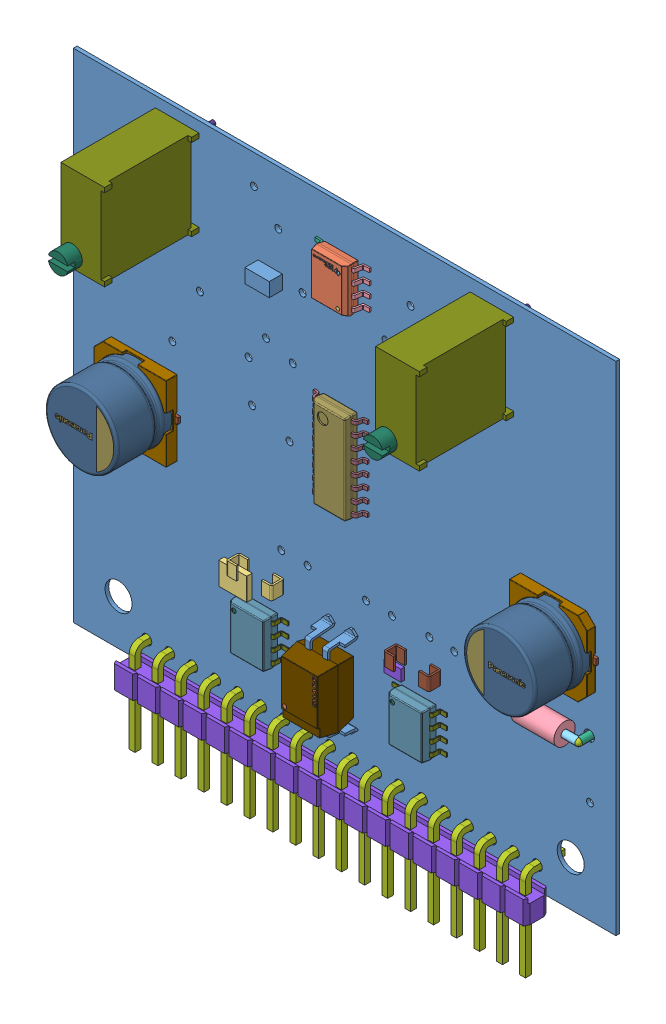
SolidWorks assembly PWM_controller, configuration Default. Lengths in mm.
Overall size (60 62.62 16.05).
432 component instances, 52 part files, 0 mates.
Components (placement in the parent):
- PWM_controller.step-2: PWM_controller.step [Default] at origin size (60 62.62 16.05)
  - Board.step-1: Board.step [Default] at origin size (60 55 0.41)
    - Open CASCADE STEP translator 6.8 2.1.1.step-1: Open CASCADE STEP translator 6.8 2.1.1.step [Default] at (0 0 -0.4115) size (60 55 0.41)
  - R32.step-1: R32.step [Default] at origin size (3.2 2.5 0.7)
    - Res_Stackpole_Electronics_RMCF1210JT5K10_eec.step-1: Res_Stackpole_Electronics_RMCF1210JT5K10_eec.step [Default] at (249.8598 58.1914 -0.4115) x (-1 0 0) z (0 0 -1) size (3.2 2.5 0.7)
      - terminals.step-1: terminals.step [Default] at origin size (3.2 2.5 0.7)
      - body.step-1: body.step [Default] at origin size (3.1 2.5 0.6)
      - top.step-1: top.step [Default] at (-0.71 0 0.65) size (2.2 2.5 0.05)
      - logo.step-1: logo.step [Default] at (0 0 0.7) size (1.25 0.57 0)
  - C2.step-1: C2.step [Default] at origin size (2.7 3.4 1)
    - 6948496496.step-1: 6948496496.step [Default] at (219.9386 58.9514 -1.4115) size (2.7 0.5 1)
      - Extruded.step-1: Extruded.step [Default] at origin size (2.7 0.5 1)
    - 6948496496.step-2: 6948496496.step [Default] at (219.9386 61.8514 -1.4115) size (2.7 0.5 1)
      - Extruded.step-1: Extruded.step [Default] at origin size (2.7 0.5 1)
    - 6948486416.step-1: 6948486416.step [Default] at (219.9386 60.4014 -1.4115) size (2.7 2.4 1)
      - Extruded-0.step-1: Extruded-0.step [Default] at origin size (2.7 2.4 1)
  - C1.step-1: C1.step [Default] at origin size (2.7 3.4 1)
    - 6948496496.step-1: 6948496496.step [Default] at (237.0328 57.9862 -1.4115) size (2.7 0.5 1)
      - Extruded.step-1: Extruded.step [Default] at origin size (2.7 0.5 1)
    - 6948496496.step-2: 6948496496.step [Default] at (237.0328 60.8862 -1.4115) size (2.7 0.5 1)
      - Extruded.step-1: Extruded.step [Default] at origin size (2.7 0.5 1)
    - 6948486416.step-1: 6948486416.step [Default] at (237.0328 59.4362 -1.4115) size (2.7 2.4 1)
      - Extruded-0.step-1: Extruded-0.step [Default] at origin size (2.7 2.4 1)
  - R31.step-1: R31.step [Default] at origin size (1.25 2 0.5)
    - Res_Vishay_CRCW0805100KFKEA_eec.step-1: Res_Vishay_CRCW0805100KFKEA_eec.step [Default] at (205.232 89.4842 -0.4115) x (0 1 0) z (0 0 -1) size (2 1.25 0.5)
      - body-1.step-1: body-1.step [Default] at (0 0 0.45) x (1 0 0) z (0 0 -1) size (1.9 1.25 0.4)
      - pad.step-1: pad.step [Default] at (-0.8133 -0.625 0.5) x (1 0 0) z (0 1 0) size (0.3 0.5 1.25)
      - pad.step-2: pad.step [Default] at (0.8133 0.625 0.5) x (-1 0 0) z (0 -1 0) size (0.3 0.5 1.25)
      - top-2.step-1: top-2.step [Default] at (0 0 0.05) x (1 0 0) z (0 0 -1) size (1.4 1.25 0.05)
      - top-2.step-2: top-2.step [Default] at (0 0 0.5) x (1 0 0) z (0 0 -1) size (1.4 1.25 0.05)
      - Vishay.step-1: Vishay.step [Default] at (0.032 -0.7832 0.5) size (0.44 0.37 0)
  - R4.step-1: R4.step [Default] at origin size (1.25 2 0.5)
    - Res_Vishay_CRCW0805100KFKEA_eec.step-1: Res_Vishay_CRCW0805100KFKEA_eec.step [Default] at (206.9846 87.503 -0.4115) x (0 -1 0) z (0 0 -1) size (2 1.25 0.5)
      - body-1.step-1: body-1.step [Default] at (0 0 0.45) x (1 0 0) z (0 0 -1) size (1.9 1.25 0.4)
      - pad.step-1: pad.step [Default] at (-0.8133 -0.625 0.5) x (1 0 0) z (0 1 0) size (0.3 0.5 1.25)
      - pad.step-2: pad.step [Default] at (0.8133 0.625 0.5) x (-1 0 0) z (0 -1 0) size (0.3 0.5 1.25)
      - top-2.step-1: top-2.step [Default] at (0 0 0.05) x (1 0 0) z (0 0 -1) size (1.4 1.25 0.05)
      - top-2.step-2: top-2.step [Default] at (0 0 0.5) x (1 0 0) z (0 0 -1) size (1.4 1.25 0.05)
      - Vishay.step-1: Vishay.step [Default] at (0.032 -0.7832 0.5) size (0.44 0.37 0)
  - R3.step-1: R3.step [Default] at origin size (1.25 2 0.5)
    - Res_Vishay_CRCW0805100KFKEA_eec.step-1: Res_Vishay_CRCW0805100KFKEA_eec.step [Default] at (210.3628 76.8604 -0.4115) x (0 -1 0) z (0 0 -1) size (2 1.25 0.5)
      - body-1.step-1: body-1.step [Default] at (0 0 0.45) x (1 0 0) z (0 0 -1) size (1.9 1.25 0.4)
      - pad.step-1: pad.step [Default] at (-0.8133 -0.625 0.5) x (1 0 0) z (0 1 0) size (0.3 0.5 1.25)
      - pad.step-2: pad.step [Default] at (0.8133 0.625 0.5) x (-1 0 0) z (0 -1 0) size (0.3 0.5 1.25)
      - top-2.step-1: top-2.step [Default] at (0 0 0.05) x (1 0 0) z (0 0 -1) size (1.4 1.25 0.05)
      - top-2.step-2: top-2.step [Default] at (0 0 0.5) x (1 0 0) z (0 0 -1) size (1.4 1.25 0.05)
      - Vishay.step-1: Vishay.step [Default] at (0.032 -0.7832 0.5) size (0.44 0.37 0)
  - R2.step-1: R2.step [Default] at origin size (1.25 2 0.5)
    - Res_Vishay_CRCW0805100KFKEA_eec.step-1: Res_Vishay_CRCW0805100KFKEA_eec.step [Default] at (223.7232 76.7588 -0.4115) x (0 -1 0) z (0 0 -1) size (2 1.25 0.5)
      - body-1.step-1: body-1.step [Default] at (0 0 0.45) x (1 0 0) z (0 0 -1) size (1.9 1.25 0.4)
      - pad.step-1: pad.step [Default] at (-0.8133 -0.625 0.5) x (1 0 0) z (0 1 0) size (0.3 0.5 1.25)
      - pad.step-2: pad.step [Default] at (0.8133 0.625 0.5) x (-1 0 0) z (0 -1 0) size (0.3 0.5 1.25)
      - top-2.step-1: top-2.step [Default] at (0 0 0.05) x (1 0 0) z (0 0 -1) size (1.4 1.25 0.05)
      - top-2.step-2: top-2.step [Default] at (0 0 0.5) x (1 0 0) z (0 0 -1) size (1.4 1.25 0.05)
      - Vishay.step-1: Vishay.step [Default] at (0.032 -0.7832 0.5) size (0.44 0.37 0)
  - R1.step-1: R1.step [Default] at origin size (1.25 2 0.5)
    - Res_Vishay_CRCW0805100KFKEA_eec.step-1: Res_Vishay_CRCW0805100KFKEA_eec.step [Default] at (225.7044 76.7842 -0.4115) x (0 1 0) z (0 0 -1) size (2 1.25 0.5)
      - body-1.step-1: body-1.step [Default] at (0 0 0.45) x (1 0 0) z (0 0 -1) size (1.9 1.25 0.4)
      - pad.step-1: pad.step [Default] at (-0.8133 -0.625 0.5) x (1 0 0) z (0 1 0) size (0.3 0.5 1.25)
      - pad.step-2: pad.step [Default] at (0.8133 0.625 0.5) x (-1 0 0) z (0 -1 0) size (0.3 0.5 1.25)
      - top-2.step-1: top-2.step [Default] at (0 0 0.05) x (1 0 0) z (0 0 -1) size (1.4 1.25 0.05)
      - top-2.step-2: top-2.step [Default] at (0 0 0.5) x (1 0 0) z (0 0 -1) size (1.4 1.25 0.05)
      - Vishay.step-1: Vishay.step [Default] at (0.032 -0.7832 0.5) size (0.44 0.37 0)
  - R30.step-1: R30.step [Default] at origin size (1.25 2 0.5)
    - Res_Vishay_CRCW0805100KFKEA_eec.step-1: Res_Vishay_CRCW0805100KFKEA_eec.step [Default] at (220.9546 82.6008 -0.4115) x (0 -1 0) z (0 0 -1) size (2 1.25 0.5)
      - body-1.step-1: body-1.step [Default] at (0 0 0.45) x (1 0 0) z (0 0 -1) size (1.9 1.25 0.4)
      - pad.step-1: pad.step [Default] at (-0.8133 -0.625 0.5) x (1 0 0) z (0 1 0) size (0.3 0.5 1.25)
      - pad.step-2: pad.step [Default] at (0.8133 0.625 0.5) x (-1 0 0) z (0 -1 0) size (0.3 0.5 1.25)
      - top-2.step-1: top-2.step [Default] at (0 0 0.05) x (1 0 0) z (0 0 -1) size (1.4 1.25 0.05)
      - top-2.step-2: top-2.step [Default] at (0 0 0.5) x (1 0 0) z (0 0 -1) size (1.4 1.25 0.05)
      - Vishay.step-1: Vishay.step [Default] at (0.032 -0.7832 0.5) size (0.44 0.37 0)
  - R29.step-1: R29.step [Default] at origin size (1.25 2 0.5)
    - Res_Vishay_CRCW0805100KFKEA_eec.step-1: Res_Vishay_CRCW0805100KFKEA_eec.step [Default] at (211.2772 90.4084 -0.4115) x (0 -1 0) z (0 0 -1) size (2 1.25 0.5)
      - body-1.step-1: body-1.step [Default] at (0 0 0.45) x (1 0 0) z (0 0 -1) size (1.9 1.25 0.4)
      - pad.step-1: pad.step [Default] at (-0.8133 -0.625 0.5) x (1 0 0) z (0 1 0) size (0.3 0.5 1.25)
      - pad.step-2: pad.step [Default] at (0.8133 0.625 0.5) x (-1 0 0) z (0 -1 0) size (0.3 0.5 1.25)
      - top-2.step-1: top-2.step [Default] at (0 0 0.05) x (1 0 0) z (0 0 -1) size (1.4 1.25 0.05)
      - top-2.step-2: top-2.step [Default] at (0 0 0.5) x (1 0 0) z (0 0 -1) size (1.4 1.25 0.05)
      - Vishay.step-1: Vishay.step [Default] at (0.032 -0.7832 0.5) size (0.44 0.37 0)
  - R28.step-1: R28.step [Default] at origin size (2 1.25 0.5)
    - Res_Vishay_CRCW0805100KFKEA_eec.step-1: Res_Vishay_CRCW0805100KFKEA_eec.step [Default] at (224.0026 85.6742 -0.4115) x (-1 0 0) z (0 0 -1) size (2 1.25 0.5)
      - body-1.step-1: body-1.step [Default] at (0 0 0.45) x (1 0 0) z (0 0 -1) size (1.9 1.25 0.4)
      - pad.step-1: pad.step [Default] at (-0.8133 -0.625 0.5) x (1 0 0) z (0 1 0) size (0.3 0.5 1.25)
      - pad.step-2: pad.step [Default] at (0.8133 0.625 0.5) x (-1 0 0) z (0 -1 0) size (0.3 0.5 1.25)
      - top-2.step-1: top-2.step [Default] at (0 0 0.05) x (1 0 0) z (0 0 -1) size (1.4 1.25 0.05)
      - top-2.step-2: top-2.step [Default] at (0 0 0.5) x (1 0 0) z (0 0 -1) size (1.4 1.25 0.05)
      - Vishay.step-1: Vishay.step [Default] at (0.032 -0.7832 0.5) size (0.44 0.37 0)
  - R27.step-1: R27.step [Default] at origin size (1.25 2 0.5)
    - Res_Vishay_CRCW0805100KFKEA_eec.step-1: Res_Vishay_CRCW0805100KFKEA_eec.step [Default] at (213.7156 87.5792 -0.4115) x (0 -1 0) z (0 0 -1) size (2 1.25 0.5)
      - body-1.step-1: body-1.step [Default] at (0 0 0.45) x (1 0 0) z (0 0 -1) size (1.9 1.25 0.4)
      - pad.step-1: pad.step [Default] at (-0.8133 -0.625 0.5) x (1 0 0) z (0 1 0) size (0.3 0.5 1.25)
      - pad.step-2: pad.step [Default] at (0.8133 0.625 0.5) x (-1 0 0) z (0 -1 0) size (0.3 0.5 1.25)
      - top-2.step-1: top-2.step [Default] at (0 0 0.05) x (1 0 0) z (0 0 -1) size (1.4 1.25 0.05)
      - top-2.step-2: top-2.step [Default] at (0 0 0.5) x (1 0 0) z (0 0 -1) size (1.4 1.25 0.05)
      - Vishay.step-1: Vishay.step [Default] at (0.032 -0.7832 0.5) size (0.44 0.37 0)
  - C14.step-1: C14.step [Default] at origin size (1.25 2 0.88)
    - Cap_KEMET_C0805C472J3HAC_eec.step-1: Cap_KEMET_C0805C472J3HAC_eec.step [Default] at (211.2264 84.3788 -0.4115) x (0 1 0) z (0 0 -1) size (1 1.15 0.78)
    - Cap_KEMET_C0805C472J3HAC_eec-3.step-1: Cap_KEMET_C0805C472J3HAC_eec-3.step [Default] at (211.2264 84.3788 -0.4115) x (0 1 0) z (0 0 -1) size (2 1.25 0.88)
    - Cap_KEMET_C0805C472J3HAC_eec-4.step-1: Cap_KEMET_C0805C472J3HAC_eec-4.step [Default] at (211.2264 84.3788 -0.4115) x (0 1 0) z (0 0 -1) size (0.59 0.12 0)
  - C13.step-1: C13.step [Default] at origin size (1.25 2 0.88)
    - Cap_KEMET_C0805C472J3HAC_eec.step-1: Cap_KEMET_C0805C472J3HAC_eec.step [Default] at (213.6648 84.3788 -0.4115) x (0 -1 0) z (0 0 -1) size (1 1.15 0.78)
    - Cap_KEMET_C0805C472J3HAC_eec-3.step-1: Cap_KEMET_C0805C472J3HAC_eec-3.step [Default] at (213.6648 84.3788 -0.4115) x (0 -1 0) z (0 0 -1) size (2 1.25 0.88)
    - Cap_KEMET_C0805C472J3HAC_eec-4.step-1: Cap_KEMET_C0805C472J3HAC_eec-4.step [Default] at (213.6648 84.3788 -0.4115) x (0 -1 0) z (0 0 -1) size (0.59 0.12 0)
  - R21.step-1: R21.step [Default] at origin size (2 1.25 0.5)
    - Res_Vishay_CRCW0805100KFKEA_eec.step-1: Res_Vishay_CRCW0805100KFKEA_eec.step [Default] at (225.0694 92.8624 -0.4115) x (1 0 0) z (0 0 -1) size (2 1.25 0.5)
      - body-1.step-1: body-1.step [Default] at (0 0 0.45) x (1 0 0) z (0 0 -1) size (1.9 1.25 0.4)
      - pad.step-1: pad.step [Default] at (-0.8133 -0.625 0.5) x (1 0 0) z (0 1 0) size (0.3 0.5 1.25)
      - pad.step-2: pad.step [Default] at (0.8133 0.625 0.5) x (-1 0 0) z (0 -1 0) size (0.3 0.5 1.25)
      - top-2.step-1: top-2.step [Default] at (0 0 0.05) x (1 0 0) z (0 0 -1) size (1.4 1.25 0.05)
      - top-2.step-2: top-2.step [Default] at (0 0 0.5) x (1 0 0) z (0 0 -1) size (1.4 1.25 0.05)
      - Vishay.step-1: Vishay.step [Default] at (0.032 -0.7832 0.5) size (0.44 0.37 0)
  - R20.step-1: R20.step [Default] at origin size (1.25 2 0.5)
    - Res_Vishay_CRCW0805100KFKEA_eec.step-1: Res_Vishay_CRCW0805100KFKEA_eec.step [Default] at (216.7382 97.3074 -0.4115) x (0 -1 0) z (0 0 -1) size (2 1.25 0.5)
      - body-1.step-1: body-1.step [Default] at (0 0 0.45) x (1 0 0) z (0 0 -1) size (1.9 1.25 0.4)
      - pad.step-1: pad.step [Default] at (-0.8133 -0.625 0.5) x (1 0 0) z (0 1 0) size (0.3 0.5 1.25)
      - pad.step-2: pad.step [Default] at (0.8133 0.625 0.5) x (-1 0 0) z (0 -1 0) size (0.3 0.5 1.25)
      - top-2.step-1: top-2.step [Default] at (0 0 0.05) x (1 0 0) z (0 0 -1) size (1.4 1.25 0.05)
      - top-2.step-2: top-2.step [Default] at (0 0 0.5) x (1 0 0) z (0 0 -1) size (1.4 1.25 0.05)
      - Vishay.step-1: Vishay.step [Default] at (0.032 -0.7832 0.5) size (0.44 0.37 0)
  - R19.step-1: R19.step [Default] at origin size (4.83 9.53 16.05)
    - Res_Bourns_3296W-1-504LF_eec.step-1: Res_Bourns_3296W-1-504LF_eec.step [Default] at (210.3653 92.9274 10.0159) x (0 0 -1) z (-1 0 0) size (1.59 2.18 2.18)
    - Res_Bourns_3296W-1-504LF_eec-5.step-1: Res_Bourns_3296W-1-504LF_eec-5.step [Default] at (210.3653 92.9274 10.0159) x (0 0 -1) z (-1 0 0) size (10.46 9.53 4.83)
    - Res_Bourns_3296W-1-504LF_eec-6.step-1: Res_Bourns_3296W-1-504LF_eec-6.step [Default] at (210.3653 92.9274 10.0159) x (0 0 -1) z (-1 0 0) size (4.53 5.59 0.51)
    - Res_Bourns_3296W-1-504LF_eec-7.step-1: Res_Bourns_3296W-1-504LF_eec-7.step [Default] at (210.3653 92.9274 10.0159) x (0 0 -1) z (-1 0 0) size (0.78 6.02 0.01)
  - R18.step-1: R18.step [Default] at origin size (1.25 2 0.5)
    - Res_Vishay_CRCW0805100KFKEA_eec.step-1: Res_Vishay_CRCW0805100KFKEA_eec.step [Default] at (214.884 97.3328 -0.4115) x (0 -1 0) z (0 0 -1) size (2 1.25 0.5)
      - body-1.step-1: body-1.step [Default] at (0 0 0.45) x (1 0 0) z (0 0 -1) size (1.9 1.25 0.4)
      - pad.step-1: pad.step [Default] at (-0.8133 -0.625 0.5) x (1 0 0) z (0 1 0) size (0.3 0.5 1.25)
      - pad.step-2: pad.step [Default] at (0.8133 0.625 0.5) x (-1 0 0) z (0 -1 0) size (0.3 0.5 1.25)
      - top-2.step-1: top-2.step [Default] at (0 0 0.05) x (1 0 0) z (0 0 -1) size (1.4 1.25 0.05)
      - top-2.step-2: top-2.step [Default] at (0 0 0.5) x (1 0 0) z (0 0 -1) size (1.4 1.25 0.05)
      - Vishay.step-1: Vishay.step [Default] at (0.032 -0.7832 0.5) size (0.44 0.37 0)
  - R17.step-1: R17.step [Default] at origin size (2 1.25 0.5)
    - Res_Vishay_CRCW0805100KFKEA_eec.step-1: Res_Vishay_CRCW0805100KFKEA_eec.step [Default] at (222.631 97.6376 -0.4115) x (-1 0 0) z (0 0 -1) size (2 1.25 0.5)
      - body-1.step-1: body-1.step [Default] at (0 0 0.45) x (1 0 0) z (0 0 -1) size (1.9 1.25 0.4)
      - pad.step-1: pad.step [Default] at (-0.8133 -0.625 0.5) x (1 0 0) z (0 1 0) size (0.3 0.5 1.25)
      - pad.step-2: pad.step [Default] at (0.8133 0.625 0.5) x (-1 0 0) z (0 -1 0) size (0.3 0.5 1.25)
      - top-2.step-1: top-2.step [Default] at (0 0 0.05) x (1 0 0) z (0 0 -1) size (1.4 1.25 0.05)
      - top-2.step-2: top-2.step [Default] at (0 0 0.5) x (1 0 0) z (0 0 -1) size (1.4 1.25 0.05)
      - Vishay.step-1: Vishay.step [Default] at (0.032 -0.7832 0.5) size (0.44 0.37 0)
  - D5.step-1: D5.step [Default] at origin size (2.7 1.55 1.45)
    - 6038362448.step-1: 6038362448.step [Default] at (235.0262 92.964 0) size (2.7 1.55 1.45)
      - Extruded-8.step-1: Extruded-8.step [Default] at origin size (2.7 1.55 1.45)
  - D4.step-1: D4.step [Default] at origin size (2.7 1.55 1.45)
    - 6038362448.step-1: 6038362448.step [Default] at (218.6178 92.7862 0) size (2.7 1.55 1.45)
      - Extruded-8.step-1: Extruded-8.step [Default] at origin size (2.7 1.55 1.45)
  - C12.step-1: C12.step [Default] at origin size (2 1.25 0.88)
    - Cap_KEMET_C0805C472J3HAC_eec.step-1: Cap_KEMET_C0805C472J3HAC_eec.step [Default] at (237.2614 97.9424 -0.4115) x (1 0 0) z (0 0 -1) size (1 1.15 0.78)
    - Cap_KEMET_C0805C472J3HAC_eec-3.step-1: Cap_KEMET_C0805C472J3HAC_eec-3.step [Default] at (237.2614 97.9424 -0.4115) x (1 0 0) z (0 0 -1) size (2 1.25 0.88)
    - Cap_KEMET_C0805C472J3HAC_eec-4.step-1: Cap_KEMET_C0805C472J3HAC_eec-4.step [Default] at (237.2614 97.9424 -0.4115) x (1 0 0) z (0 0 -1) size (0.59 0.12 0)
  - C11.step-1: C11.step [Default] at origin size (1.25 2 0.88)
    - Cap_KEMET_C0805C472J3HAC_eec.step-1: Cap_KEMET_C0805C472J3HAC_eec.step [Default] at (212.6996 97.3836 -0.4115) x (0 -1 0) z (0 0 -1) size (1 1.15 0.78)
    - Cap_KEMET_C0805C472J3HAC_eec-3.step-1: Cap_KEMET_C0805C472J3HAC_eec-3.step [Default] at (212.6996 97.3836 -0.4115) x (0 -1 0) z (0 0 -1) size (2 1.25 0.88)
    - Cap_KEMET_C0805C472J3HAC_eec-4.step-1: Cap_KEMET_C0805C472J3HAC_eec-4.step [Default] at (212.6996 97.3836 -0.4115) x (0 -1 0) z (0 0 -1) size (0.59 0.12 0)
  - R25.step-1: R25.step [Default] at origin size (2 1.25 0.5)
    - Res_Vishay_CRCW0805100KFKEA_eec.step-1: Res_Vishay_CRCW0805100KFKEA_eec.step [Default] at (231.2416 97.663 -0.4115) x (-1 0 0) z (0 0 -1) size (2 1.25 0.5)
      - body-1.step-1: body-1.step [Default] at (0 0 0.45) x (1 0 0) z (0 0 -1) size (1.9 1.25 0.4)
      - pad.step-1: pad.step [Default] at (-0.8133 -0.625 0.5) x (1 0 0) z (0 1 0) size (0.3 0.5 1.25)
      - pad.step-2: pad.step [Default] at (0.8133 0.625 0.5) x (-1 0 0) z (0 -1 0) size (0.3 0.5 1.25)
      - top-2.step-1: top-2.step [Default] at (0 0 0.05) x (1 0 0) z (0 0 -1) size (1.4 1.25 0.05)
      - top-2.step-2: top-2.step [Default] at (0 0 0.5) x (1 0 0) z (0 0 -1) size (1.4 1.25 0.05)
      - Vishay.step-1: Vishay.step [Default] at (0.032 -0.7832 0.5) size (0.44 0.37 0)
  - R23.step-1: R23.step [Default] at origin size (2 1.25 0.5)
    - Res_Vishay_CRCW0805100KFKEA_eec.step-1: Res_Vishay_CRCW0805100KFKEA_eec.step [Default] at (237.2614 100.1268 -0.4115) x (1 0 0) z (0 0 -1) size (2 1.25 0.5)
      - body-1.step-1: body-1.step [Default] at (0 0 0.45) x (1 0 0) z (0 0 -1) size (1.9 1.25 0.4)
      - pad.step-1: pad.step [Default] at (-0.8133 -0.625 0.5) x (1 0 0) z (0 1 0) size (0.3 0.5 1.25)
      - pad.step-2: pad.step [Default] at (0.8133 0.625 0.5) x (-1 0 0) z (0 -1 0) size (0.3 0.5 1.25)
      - top-2.step-1: top-2.step [Default] at (0 0 0.05) x (1 0 0) z (0 0 -1) size (1.4 1.25 0.05)
      - top-2.step-2: top-2.step [Default] at (0 0 0.5) x (1 0 0) z (0 0 -1) size (1.4 1.25 0.05)
      - Vishay.step-1: Vishay.step [Default] at (0.032 -0.7832 0.5) size (0.44 0.37 0)
  - R26.step-1: R26.step [Default] at origin size (2 1.25 0.5)
    - Res_Vishay_CRCW0805100KFKEA_eec.step-1: Res_Vishay_CRCW0805100KFKEA_eec.step [Default] at (228.6508 92.8624 -0.4115) x (-1 0 0) z (0 0 -1) size (2 1.25 0.5)
      - body-1.step-1: body-1.step [Default] at (0 0 0.45) x (1 0 0) z (0 0 -1) size (1.9 1.25 0.4)
      - pad.step-1: pad.step [Default] at (-0.8133 -0.625 0.5) x (1 0 0) z (0 1 0) size (0.3 0.5 1.25)
      - pad.step-2: pad.step [Default] at (0.8133 0.625 0.5) x (-1 0 0) z (0 -1 0) size (0.3 0.5 1.25)
      - top-2.step-1: top-2.step [Default] at (0 0 0.05) x (1 0 0) z (0 0 -1) size (1.4 1.25 0.05)
      - top-2.step-2: top-2.step [Default] at (0 0 0.5) x (1 0 0) z (0 0 -1) size (1.4 1.25 0.05)
      - Vishay.step-1: Vishay.step [Default] at (0.032 -0.7832 0.5) size (0.44 0.37 0)
  - R22.step-1: R22.step [Default] at origin size (2 1.25 0.5)
    - Res_Vishay_CRCW0805100KFKEA_eec.step-1: Res_Vishay_CRCW0805100KFKEA_eec.step [Default] at (234.2388 95.2754 -0.4115) x (1 0 0) z (0 0 -1) size (2 1.25 0.5)
      - body-1.step-1: body-1.step [Default] at (0 0 0.45) x (1 0 0) z (0 0 -1) size (1.9 1.25 0.4)
      - pad.step-1: pad.step [Default] at (-0.8133 -0.625 0.5) x (1 0 0) z (0 1 0) size (0.3 0.5 1.25)
      - pad.step-2: pad.step [Default] at (0.8133 0.625 0.5) x (-1 0 0) z (0 -1 0) size (0.3 0.5 1.25)
      - top-2.step-1: top-2.step [Default] at (0 0 0.05) x (1 0 0) z (0 0 -1) size (1.4 1.25 0.05)
      - top-2.step-2: top-2.step [Default] at (0 0 0.5) x (1 0 0) z (0 0 -1) size (1.4 1.25 0.05)
      - Vishay.step-1: Vishay.step [Default] at (0.032 -0.7832 0.5) size (0.44 0.37 0)
  - R24.step-1: R24.step [Default] at origin size (4.83 9.53 16.05)
    - Res_Bourns_3296W-1-504LF_eec.step-1: Res_Bourns_3296W-1-504LF_eec.step [Default] at (245.1683 92.6988 10.0159) x (0 0 -1) z (-1 0 0) size (1.59 2.18 2.18)
    - Res_Bourns_3296W-1-504LF_eec-5.step-1: Res_Bourns_3296W-1-504LF_eec-5.step [Default] at (245.1683 92.6988 10.0159) x (0 0 -1) z (-1 0 0) size (10.46 9.53 4.83)
    - Res_Bourns_3296W-1-504LF_eec-6.step-1: Res_Bourns_3296W-1-504LF_eec-6.step [Default] at (245.1683 92.6988 10.0159) x (0 0 -1) z (-1 0 0) size (4.53 5.59 0.51)
    - Res_Bourns_3296W-1-504LF_eec-7.step-1: Res_Bourns_3296W-1-504LF_eec-7.step [Default] at (245.1683 92.6988 10.0159) x (0 0 -1) z (-1 0 0) size (0.78 6.02 0.01)
  - U4.step-1: U4.step [Default] at origin size (6 4.9 1.76)
    - IC_Texas_Instruments_ISO7220ADR_eec.step-1: IC_Texas_Instruments_ISO7220ADR_eec.step [Default] at (226.7712 96.9772 0) x (-1 0 0) z (0 0 1) size (6 4.9 1.76)
      - IC_BODY.step-1: IC_BODY.step [Default] at (0 0 0.25) x (0 -1 0) z (0 0 1) size (4.9 3.9 1.5)
      - circle.step-1: circle.step [Default] at (-1.0726 1.9393 1.751) x (1 0 0) z (0 0 -1) size (0.4 0.4 0)
      - IC_LEG.step-1: IC_LEG.step [Default] at (-3 2.1095 0) x (1 0 0) z (0 -1 0) size (1.15 1.11 0.41)
      - IC_LEG.step-2: IC_LEG.step [Default] at (-3 0.8395 0) x (1 0 0) z (0 -1 0) size (1.15 1.11 0.41)
      - IC_LEG.step-3: IC_LEG.step [Default] at (-3 -0.4305 0) x (1 0 0) z (0 -1 0) size (1.15 1.11 0.41)
      - IC_LEG.step-4: IC_LEG.step [Default] at (-3 -1.7005 0) x (1 0 0) z (0 -1 0) size (1.15 1.11 0.41)
      - Texas_Instruments.step-1: Texas_Instruments.step [Default] at (0.0232 -1.7093 1.75) size (3.04 0.71 0.02)
      - IC_LEG_MIR8.step-1: IC_LEG_MIR8.step [Default] at (3 2.1095 0) x (-1 0 0) z (0 1 0) size (1.15 1.11 0.41)
      - IC_LEG_MIR8.step-2: IC_LEG_MIR8.step [Default] at (3 0.8395 0) x (-1 0 0) z (0 1 0) size (1.15 1.11 0.41)
      - IC_LEG_MIR8.step-3: IC_LEG_MIR8.step [Default] at (3 -0.4305 0) x (-1 0 0) z (0 1 0) size (1.15 1.11 0.41)
      - IC_LEG_MIR8.step-4: IC_LEG_MIR8.step [Default] at (3 -1.7005 0) x (-1 0 0) z (0 1 0) size (1.15 1.11 0.41)
  - P2.step-1: P2.step [Default] at origin size (45.72 10.36 5.54)
    - 61301811021.step-1: 61301811021.step [Default] at (226.5681 48.2841 1.31) x (-1 0 0) z (0 -1 0) size (45.72 5.54 10.36)
      - 6130xx11021_PIN.step-1: 6130xx11021_PIN.step [Default] at (-21.59 0 2.09) size (0.64 4.59 10.36)
      - 6130xx11021_PIN.step-2: 6130xx11021_PIN.step [Default] at (-19.05 0 2.09) size (0.64 4.59 10.36)
      - 6130xx11021_PIN.step-3: 6130xx11021_PIN.step [Default] at (-16.51 0 2.09) size (0.64 4.59 10.36)
      - 6130xx11021_PIN.step-4: 6130xx11021_PIN.step [Default] at (-13.97 0 2.09) size (0.64 4.59 10.36)
      - 6130xx11021_PIN.step-5: 6130xx11021_PIN.step [Default] at (-11.43 0 2.09) size (0.64 4.59 10.36)
      - 6130xx11021_PIN.step-6: 6130xx11021_PIN.step [Default] at (-8.89 0 2.09) size (0.64 4.59 10.36)
      - 6130xx11021_PIN.step-7: 6130xx11021_PIN.step [Default] at (-6.35 0 2.09) size (0.64 4.59 10.36)
      - 6130xx11021_PIN.step-8: 6130xx11021_PIN.step [Default] at (-3.81 0 2.09) size (0.64 4.59 10.36)
      - 6130xx11021_PIN.step-9: 6130xx11021_PIN.step [Default] at (-1.27 0 2.09) size (0.64 4.59 10.36)
      - 6130xx11021_PIN.step-10: 6130xx11021_PIN.step [Default] at (1.27 0 2.09) size (0.64 4.59 10.36)
      - 6130xx11021_PIN.step-11: 6130xx11021_PIN.step [Default] at (3.81 0 2.09) size (0.64 4.59 10.36)
      - 6130xx11021_PIN.step-12: 6130xx11021_PIN.step [Default] at (6.35 0 2.09) size (0.64 4.59 10.36)
      - 6130xx11021_PIN.step-13: 6130xx11021_PIN.step [Default] at (8.89 0 2.09) size (0.64 4.59 10.36)
      - 6130xx11021_PIN.step-14: 6130xx11021_PIN.step [Default] at (11.43 0 2.09) size (0.64 4.59 10.36)
      - 6130xx11021_PIN.step-15: 6130xx11021_PIN.step [Default] at (13.97 0 2.09) size (0.64 4.59 10.36)
      - 6130xx11021_PIN.step-16: 6130xx11021_PIN.step [Default] at (16.51 0 2.09) size (0.64 4.59 10.36)
      - 6130xx11021_PIN.step-17: 6130xx11021_PIN.step [Default] at (19.05 0 2.09) size (0.64 4.59 10.36)
      - 6130xx11021_PIN.step-18: 6130xx11021_PIN.step [Default] at (21.59 0 2.09) size (0.64 4.59 10.36)
      - 61301811021-9.step-1: 61301811021-9.step [Default] at origin size (45.72 2.54 2.54)
  - R5.step-1: R5.step [Default] at origin size (1.25 2 0.5)
    - Res_Vishay_CRCW0805100KFKEA_eec.step-1: Res_Vishay_CRCW0805100KFKEA_eec.step [Default] at (208.788 84.3378 -0.4115) x (0 -1 0) z (0 0 -1) size (2 1.25 0.5)
      - body-1.step-1: body-1.step [Default] at (0 0 0.45) x (1 0 0) z (0 0 -1) size (1.9 1.25 0.4)
      - pad.step-1: pad.step [Default] at (-0.8133 -0.625 0.5) x (1 0 0) z (0 1 0) size (0.3 0.5 1.25)
      - pad.step-2: pad.step [Default] at (0.8133 0.625 0.5) x (-1 0 0) z (0 -1 0) size (0.3 0.5 1.25)
      - top-2.step-1: top-2.step [Default] at (0 0 0.05) x (1 0 0) z (0 0 -1) size (1.4 1.25 0.05)
      - top-2.step-2: top-2.step [Default] at (0 0 0.5) x (1 0 0) z (0 0 -1) size (1.4 1.25 0.05)
      - Vishay.step-1: Vishay.step [Default] at (0.032 -0.7832 0.5) size (0.44 0.37 0)
  - R9.step-1: R9.step [Default] at origin size (1.25 2 0.5)
    - Res_Vishay_CRCW0805100KFKEA_eec.step-1: Res_Vishay_CRCW0805100KFKEA_eec.step [Default] at (206.9592 84.328 -0.4115) x (0 1 0) z (0 0 -1) size (2 1.25 0.5)
      - body-1.step-1: body-1.step [Default] at (0 0 0.45) x (1 0 0) z (0 0 -1) size (1.9 1.25 0.4)
      - pad.step-1: pad.step [Default] at (-0.8133 -0.625 0.5) x (1 0 0) z (0 1 0) size (0.3 0.5 1.25)
      - pad.step-2: pad.step [Default] at (0.8133 0.625 0.5) x (-1 0 0) z (0 -1 0) size (0.3 0.5 1.25)
      - top-2.step-1: top-2.step [Default] at (0 0 0.05) x (1 0 0) z (0 0 -1) size (1.4 1.25 0.05)
      - top-2.step-2: top-2.step [Default] at (0 0 0.5) x (1 0 0) z (0 0 -1) size (1.4 1.25 0.05)
      - Vishay.step-1: Vishay.step [Default] at (0.032 -0.7832 0.5) size (0.44 0.37 0)
  - R6.step-1: R6.step [Default] at origin size (3.2 2.5 0.7)
    - Res_Stackpole_Electronics_RMCF1210JT5K10_eec.step-1: Res_Stackpole_Electronics_RMCF1210JT5K10_eec.step [Default] at (249.8854 61.6712 -0.4115) x (-1 0 0) z (0 0 -1) size (3.2 2.5 0.7)
      - terminals.step-1: terminals.step [Default] at origin size (3.2 2.5 0.7)
      - body.step-1: body.step [Default] at origin size (3.1 2.5 0.6)
      - top.step-1: top.step [Default] at (-0.71 0 0.65) size (2.2 2.5 0.05)
      - logo.step-1: logo.step [Default] at (0 0 0.7) size (1.25 0.57 0)
  - C5.step-1: C5.step [Default] at origin size (9 8.3 6.5)
    - Cap_Panasonic_Electronic_Components_EEE-FK1H101GP_eec.step-1: Cap_Panasonic_Electronic_Components_EEE-FK1H101GP_eec.step [Default] at (204.216 73.9902 0) x (-1 0 0) z (0 0 1) size (9 8.3 6.5)
      - base.step-1: base.step [Default] at origin size (8.3 8.3 1.25)
      - cap.step-1: cap.step [Default] at origin size (8 8 6)
      - pins.step-1: pins.step [Default] at origin size (9 0.65 0.3)
      - logo-10.step-1: logo-10.step [Default] at (0 0 6.5) size (6.48 6.34 0)
  - C6.step-1: C6.step [Default] at origin size (2.7 3.4 1)
    - 6948496496.step-1: 6948496496.step [Default] at (213.487 78.9708 -1.4115) size (2.7 0.5 1)
      - Extruded.step-1: Extruded.step [Default] at origin size (2.7 0.5 1)
    - 6948496496.step-2: 6948496496.step [Default] at (213.487 76.0708 -1.4115) size (2.7 0.5 1)
      - Extruded.step-1: Extruded.step [Default] at origin size (2.7 0.5 1)
    - 6948486416.step-1: 6948486416.step [Default] at (213.487 77.5208 -1.4115) size (2.7 2.4 1)
      - Extruded-0.step-1: Extruded-0.step [Default] at origin size (2.7 2.4 1)
  - C7.step-1: C7.step [Default] at origin size (1.25 2 0.88)
    - Cap_KEMET_C0805C472J3HAC_eec.step-1: Cap_KEMET_C0805C472J3HAC_eec.step [Default] at (216.662 76.6318 -0.4115) x (0 -1 0) z (0 0 -1) size (1 1.15 0.78)
    - Cap_KEMET_C0805C472J3HAC_eec-3.step-1: Cap_KEMET_C0805C472J3HAC_eec-3.step [Default] at (216.662 76.6318 -0.4115) x (0 -1 0) z (0 0 -1) size (2 1.25 0.88)
    - Cap_KEMET_C0805C472J3HAC_eec-4.step-1: Cap_KEMET_C0805C472J3HAC_eec-4.step [Default] at (216.662 76.6318 -0.4115) x (0 -1 0) z (0 0 -1) size (0.59 0.12 0)
  - R14.step-1: R14.step [Default] at origin size (2.5 3.2 0.6)
    - Res_Vishay_CRCW12104K70FKEC_eec.step-1: Res_Vishay_CRCW12104K70FKEC_eec.step [Default] at (209.55 54.0512 -0.4115) x (0 -1 0) z (0 0 -1) size (3.2 2.5 0.6)
      - body-11.step-1: body-11.step [Default] at (0 0 0.55) x (1 0 0) z (0 0 -1) size (3.1 2.5 0.5)
      - pad-12.step-1: pad-12.step [Default] at (-1.4133 -1.25 0.6) x (1 0 0) z (0 1 0) size (0.45 0.6 2.5)
      - pad-12.step-2: pad-12.step [Default] at (1.4133 1.25 0.6) x (-1 0 0) z (0 -1 0) size (0.45 0.6 2.5)
      - top-13.step-1: top-13.step [Default] at (0 0 0.6) x (1 0 0) z (0 0 -1) size (2.4 2.5 0.05)
      - Vishay-14.step-1: Vishay-14.step [Default] at (0.0049 -0.739 0.6) size (0.44 0.37 0)
      - bottom.step-1: bottom.step [Default] at (0 0 0.05) x (1 0 0) z (0 0 -1) size (2.3 2.5 0.05)
  - R13.step-1: R13.step [Default] at origin size (2.5 3.2 0.6)
    - Res_Vishay_CRCW12104K70FKEC_eec.step-1: Res_Vishay_CRCW12104K70FKEC_eec.step [Default] at (213.2584 54.1274 -0.4115) x (0 -1 0) z (0 0 -1) size (3.2 2.5 0.6)
      - body-11.step-1: body-11.step [Default] at (0 0 0.55) x (1 0 0) z (0 0 -1) size (3.1 2.5 0.5)
      - pad-12.step-1: pad-12.step [Default] at (-1.4133 -1.25 0.6) x (1 0 0) z (0 1 0) size (0.45 0.6 2.5)
      - pad-12.step-2: pad-12.step [Default] at (1.4133 1.25 0.6) x (-1 0 0) z (0 -1 0) size (0.45 0.6 2.5)
      - top-13.step-1: top-13.step [Default] at (0 0 0.6) x (1 0 0) z (0 0 -1) size (2.4 2.5 0.05)
      - Vishay-14.step-1: Vishay-14.step [Default] at (0.0049 -0.739 0.6) size (0.44 0.37 0)
      - bottom.step-1: bottom.step [Default] at (0 0 0.05) x (1 0 0) z (0 0 -1) size (2.3 2.5 0.05)
  - R16.step-1: R16.step [Default] at origin size (2 1.25 0.5)
    - Res_Vishay_CRCW0805100KFKEA_eec.step-1: Res_Vishay_CRCW0805100KFKEA_eec.step [Default] at (208.6004 62.611 -0.4115) x (-1 0 0) z (0 0 -1) size (2 1.25 0.5)
      - body-1.step-1: body-1.step [Default] at (0 0 0.45) x (1 0 0) z (0 0 -1) size (1.9 1.25 0.4)
      - pad.step-1: pad.step [Default] at (-0.8133 -0.625 0.5) x (1 0 0) z (0 1 0) size (0.3 0.5 1.25)
      - pad.step-2: pad.step [Default] at (0.8133 0.625 0.5) x (-1 0 0) z (0 -1 0) size (0.3 0.5 1.25)
      - top-2.step-1: top-2.step [Default] at (0 0 0.05) x (1 0 0) z (0 0 -1) size (1.4 1.25 0.05)
      - top-2.step-2: top-2.step [Default] at (0 0 0.5) x (1 0 0) z (0 0 -1) size (1.4 1.25 0.05)
      - Vishay.step-1: Vishay.step [Default] at (0.032 -0.7832 0.5) size (0.44 0.37 0)
  - R7.step-1: R7.step [Default] at origin size (1.25 2 0.5)
    - Res_Vishay_CRCW0805100KFKEA_eec.step-1: Res_Vishay_CRCW0805100KFKEA_eec.step [Default] at (232.0544 70.231 -0.4115) x (0 1 0) z (0 0 -1) size (2 1.25 0.5)
      - body-1.step-1: body-1.step [Default] at (0 0 0.45) x (1 0 0) z (0 0 -1) size (1.9 1.25 0.4)
      - pad.step-1: pad.step [Default] at (-0.8133 -0.625 0.5) x (1 0 0) z (0 1 0) size (0.3 0.5 1.25)
      - pad.step-2: pad.step [Default] at (0.8133 0.625 0.5) x (-1 0 0) z (0 -1 0) size (0.3 0.5 1.25)
      - top-2.step-1: top-2.step [Default] at (0 0 0.05) x (1 0 0) z (0 0 -1) size (1.4 1.25 0.05)
      - top-2.step-2: top-2.step [Default] at (0 0 0.5) x (1 0 0) z (0 0 -1) size (1.4 1.25 0.05)
      - Vishay.step-1: Vishay.step [Default] at (0.032 -0.7832 0.5) size (0.44 0.37 0)
  - R15.step-1: R15.step [Default] at origin size (2 1.25 0.5)
    - Res_Vishay_CRCW0805100KFKEA_eec.step-1: Res_Vishay_CRCW0805100KFKEA_eec.step [Default] at (208.6102 60.7568 -0.4115) x (-1 0 0) z (0 0 -1) size (2 1.25 0.5)
      - body-1.step-1: body-1.step [Default] at (0 0 0.45) x (1 0 0) z (0 0 -1) size (1.9 1.25 0.4)
      - pad.step-1: pad.step [Default] at (-0.8133 -0.625 0.5) x (1 0 0) z (0 1 0) size (0.3 0.5 1.25)
      - pad.step-2: pad.step [Default] at (0.8133 0.625 0.5) x (-1 0 0) z (0 -1 0) size (0.3 0.5 1.25)
      - top-2.step-1: top-2.step [Default] at (0 0 0.05) x (1 0 0) z (0 0 -1) size (1.4 1.25 0.05)
      - top-2.step-2: top-2.step [Default] at (0 0 0.5) x (1 0 0) z (0 0 -1) size (1.4 1.25 0.05)
      - Vishay.step-1: Vishay.step [Default] at (0.032 -0.7832 0.5) size (0.44 0.37 0)
  - R10.step-1: R10.step [Default] at origin size (1.25 2 0.5)
    - Res_Vishay_CRCW0805100KFKEA_eec.step-1: Res_Vishay_CRCW0805100KFKEA_eec.step [Default] at (229.2096 70.1802 -0.4115) x (0 1 0) z (0 0 -1) size (2 1.25 0.5)
      - body-1.step-1: body-1.step [Default] at (0 0 0.45) x (1 0 0) z (0 0 -1) size (1.9 1.25 0.4)
      - pad.step-1: pad.step [Default] at (-0.8133 -0.625 0.5) x (1 0 0) z (0 1 0) size (0.3 0.5 1.25)
      - pad.step-2: pad.step [Default] at (0.8133 0.625 0.5) x (-1 0 0) z (0 -1 0) size (0.3 0.5 1.25)
      - top-2.step-1: top-2.step [Default] at (0 0 0.05) x (1 0 0) z (0 0 -1) size (1.4 1.25 0.05)
      - top-2.step-2: top-2.step [Default] at (0 0 0.5) x (1 0 0) z (0 0 -1) size (1.4 1.25 0.05)
      - Vishay.step-1: Vishay.step [Default] at (0.032 -0.7832 0.5) size (0.44 0.37 0)
  - R11.step-1: R11.step [Default] at origin size (2.5 3.2 0.6)
    - Res_Vishay_CRCW12104K70FKEC_eec.step-1: Res_Vishay_CRCW12104K70FKEC_eec.step [Default] at (219.4814 54.1528 -0.4115) x (0 -1 0) z (0 0 -1) size (3.2 2.5 0.6)
      - body-11.step-1: body-11.step [Default] at (0 0 0.55) x (1 0 0) z (0 0 -1) size (3.1 2.5 0.5)
      - pad-12.step-1: pad-12.step [Default] at (-1.4133 -1.25 0.6) x (1 0 0) z (0 1 0) size (0.45 0.6 2.5)
      - pad-12.step-2: pad-12.step [Default] at (1.4133 1.25 0.6) x (-1 0 0) z (0 -1 0) size (0.45 0.6 2.5)
      - top-13.step-1: top-13.step [Default] at (0 0 0.6) x (1 0 0) z (0 0 -1) size (2.4 2.5 0.05)
      - Vishay-14.step-1: Vishay-14.step [Default] at (0.0049 -0.739 0.6) size (0.44 0.37 0)
      - bottom.step-1: bottom.step [Default] at (0 0 0.05) x (1 0 0) z (0 0 -1) size (2.3 2.5 0.05)
  - R12.step-1: R12.step [Default] at origin size (1.25 2 0.5)
    - Res_Vishay_CRCW0805100KFKEA_eec.step-1: Res_Vishay_CRCW0805100KFKEA_eec.step [Default] at (218.6686 76.7842 -0.4115) x (0 -1 0) z (0 0 -1) size (2 1.25 0.5)
      - body-1.step-1: body-1.step [Default] at (0 0 0.45) x (1 0 0) z (0 0 -1) size (1.9 1.25 0.4)
      - pad.step-1: pad.step [Default] at (-0.8133 -0.625 0.5) x (1 0 0) z (0 1 0) size (0.3 0.5 1.25)
      - pad.step-2: pad.step [Default] at (0.8133 0.625 0.5) x (-1 0 0) z (0 -1 0) size (0.3 0.5 1.25)
      - top-2.step-1: top-2.step [Default] at (0 0 0.05) x (1 0 0) z (0 0 -1) size (1.4 1.25 0.05)
      - top-2.step-2: top-2.step [Default] at (0 0 0.5) x (1 0 0) z (0 0 -1) size (1.4 1.25 0.05)
      - Vishay.step-1: Vishay.step [Default] at (0.032 -0.7832 0.5) size (0.44 0.37 0)
  - R8.step-1: R8.step [Default] at origin size (2.5 3.2 0.6)
    - Res_Vishay_CRCW12104K70FKEC_eec.step-1: Res_Vishay_CRCW12104K70FKEC_eec.step [Default] at (222.9866 54.1782 -0.4115) x (0 -1 0) z (0 0 -1) size (3.2 2.5 0.6)
      - body-11.step-1: body-11.step [Default] at (0 0 0.55) x (1 0 0) z (0 0 -1) size (3.1 2.5 0.5)
      - pad-12.step-1: pad-12.step [Default] at (-1.4133 -1.25 0.6) x (1 0 0) z (0 1 0) size (0.45 0.6 2.5)
      - pad-12.step-2: pad-12.step [Default] at (1.4133 1.25 0.6) x (-1 0 0) z (0 -1 0) size (0.45 0.6 2.5)
      - top-13.step-1: top-13.step [Default] at (0 0 0.6) x (1 0 0) z (0 0 -1) size (2.4 2.5 0.05)
      - Vishay-14.step-1: Vishay-14.step [Default] at (0.0049 -0.739 0.6) size (0.44 0.37 0)
      - bottom.step-1: bottom.step [Default] at (0 0 0.05) x (1 0 0) z (0 0 -1) size (2.3 2.5 0.05)
  - Q1.step-1: Q1.step [Default] at origin size (4.58 10 4.6)
    - Trans_SHARP_PC817XNNIP0F_eec.step-1: Trans_SHARP_PC817XNNIP0F_eec.step [Default] at (226.441 58.547 0) x (0 1 0) z (0 0 1) size (10 4.58 4.6)
      - body-15.step-1: body-15.step [Default] at origin size (6.5 4.58 4)
      - terminals-16.step-1: terminals-16.step [Default] at origin size (10 3.74 2.73)
      - logo-17.step-1: logo-17.step [Default] at (-3.25 0 4.6) size (4.76 3.7 0)
  - D3.step-1: D3.step [Default] at origin size (6.37 3.44 1.43)
    - 6010098432.step-1: 6010098432.step [Default] at (217.678 63.754 0) size (6.37 3.44 1.43)
      - body.step-1: body.step [Default] at (-2.3 -1.46 0.25) size (3.1 2.5 0.6)
      - Lead.step-1: Lead.step [Default] at (1.38 0 0) size (1.14 1.45 1.43)
      - Lead.step-2: Lead.step [Default] at (-1.38 0 0) x (-1 0 0) z (0 0 1) size (1.14 1.45 1.43)
  - D2.step-1: D2.step [Default] at origin size (8.58 2.35 4.35)
    - 5955066400.step-1: 5955066400.step [Default] at (247.6485 66.3194 1.175) x (0 0 -1) z (1 0 0) size (2.35 2.35 4.7)
      - Cylinder.step-1: Cylinder.step [Default] at origin size (2.35 2.35 4.7)
    - 5955067280.step-1: 5955067280.step [Default] at (252.348 66.3194 1.175) x (0 0 -1) z (1 0 0) size (0.79 0.79 1.55)
      - Cylinder-18.step-1: Cylinder-18.step [Default] at origin size (0.79 0.79 1.55)
    - 5955066240.step-1: 5955066240.step [Default] at (253.8982 66.3196 -2) x (1 0 0) z (0 0 1) size (0.79 0.79 3.17)
      - Cylinder-19.step-1: Cylinder-19.step [Default] at origin size (0.79 0.79 3.17)
    - 5955066160.step-1: 5955066160.step [Default] at (253.8981 66.3195 1.175) x (1 0 0) z (0 0 1) size (0.79 0.79 0.79)
      - Sphere.step-1: Sphere.step [Default] at origin size (0.79 0.79 0.79)
    - 5955066080.step-1: 5955066080.step [Default] at (246.099 66.3195 1.175) x (-1 0 0) z (0 0 1) size (0.79 0.79 0.79)
      - Sphere-20.step-1: Sphere-20.step [Default] at origin size (0.79 0.79 0.79)
    - 5955066000.step-1: 5955066000.step [Default] at (246.0989 66.3196 -2) x (-1 0 0) z (0 0 1) size (0.79 0.79 3.17)
      - Cylinder-21.step-1: Cylinder-21.step [Default] at origin size (0.79 0.79 3.17)
    - 5955065920.step-1: 5955065920.step [Default] at (247.6491 66.3194 1.175) x (0 0 -1) z (-1 0 0) size (0.79 0.79 1.55)
      - Cylinder-22.step-1: Cylinder-22.step [Default] at origin size (0.79 0.79 1.55)
  - D1.step-1: D1.step [Default] at origin size (5.77 2.81 1.43)
    - 6702799872.step-1: 6702799872.step [Default] at (235.077 63.754 0) x (1 0 0) z (0 0 1) size (5.77 2.81 1.43)
      - body-1.step-1: body-1.step [Default] at (-2.3 -1.46 0.25) size (1.9 1.25 0.4)
      - Lead-24.step-1: Lead-24.step [Default] at (1.38 0 0) size (1.14 1.45 1.43)
      - Lead-24.step-2: Lead-24.step [Default] at (-1.38 0 0) x (-1 0 0) z (0 0 1) size (1.14 1.45 1.43)
  - C8.step-1: C8.step [Default] at origin size (2.7 3.4 1)
    - 6948496496.step-1: 6948496496.step [Default] at (233.2228 57.986 -1.4115) size (2.7 0.5 1)
      - Extruded.step-1: Extruded.step [Default] at origin size (2.7 0.5 1)
    - 6948496496.step-2: 6948496496.step [Default] at (233.2228 60.886 -1.4115) size (2.7 0.5 1)
      - Extruded.step-1: Extruded.step [Default] at origin size (2.7 0.5 1)
    - 6948486416.step-1: 6948486416.step [Default] at (233.2228 59.436 -1.4115) size (2.7 2.4 1)
      - Extruded-0.step-1: Extruded-0.step [Default] at origin size (2.7 2.4 1)
  - C9.step-1: C9.step [Default] at origin size (2.7 3.4 1)
    - 6948496496.step-1: 6948496496.step [Default] at (216.154 58.9512 -1.4115) size (2.7 0.5 1)
      - Extruded.step-1: Extruded.step [Default] at origin size (2.7 0.5 1)
    - 6948496496.step-2: 6948496496.step [Default] at (216.154 61.8512 -1.4115) size (2.7 0.5 1)
      - Extruded.step-1: Extruded.step [Default] at origin size (2.7 0.5 1)
    - 6948486416.step-1: 6948486416.step [Default] at (216.154 60.4012 -1.4115) size (2.7 2.4 1)
      - Extruded-0.step-1: Extruded-0.step [Default] at origin size (2.7 2.4 1)
  - C10.step-1: C10.step [Default] at origin size (9 8.3 6.5)
    - Cap_Panasonic_Electronic_Components_EEE-FK1H101GP_eec.step-1: Cap_Panasonic_Electronic_Components_EEE-FK1H101GP_eec.step [Default] at (250.45 73.9902 0) x (1 0 0) z (0 0 1) size (9 8.3 6.5)
      - base.step-1: base.step [Default] at origin size (8.3 8.3 1.25)
      - cap.step-1: cap.step [Default] at origin size (8 8 6)
      - pins.step-1: pins.step [Default] at origin size (9 0.65 0.3)
      - logo-10.step-1: logo-10.step [Default] at (0 0 6.5) size (6.48 6.34 0)
  - U1.step-1: U1.step [Default] at origin size (5.99 9.91 1.6)
    - SOIC-16akaD0016AakaM16A.step-1: SOIC-16akaD0016AakaM16A.step [Default] at (226.5679 79.7559 0.97) x (0 -1 0) z (-1 0 0) size (9.91 1.6 5.99)
      - M16A_ASM_24_ASM.step-1: M16A_ASM_24_ASM.step [Default] at origin size (9.91 1.6 5.99)
        - BODY_M16A_17.step-1: BODY_M16A_17.step [Default] at origin size (9.91 1.45 3.92)
        - LEAD_M16A_42.step-1: LEAD_M16A_42.step [Default] at (4.445 -0.6223 2.348) size (0.37 0.98 1.04)
        - LEAD_M16A_42.step-2: LEAD_M16A_42.step [Default] at (3.175 -0.6223 2.348) size (0.37 0.98 1.04)
        - LEAD_M16A_42.step-3: LEAD_M16A_42.step [Default] at (1.905 -0.6223 2.348) size (0.37 0.98 1.04)
        - LEAD_M16A_42.step-4: LEAD_M16A_42.step [Default] at (0.635 -0.6223 2.348) size (0.37 0.98 1.04)
        - LEAD_M16A_42.step-5: LEAD_M16A_42.step [Default] at (-0.635 -0.6223 2.348) size (0.37 0.98 1.04)
        - LEAD_M16A_42.step-6: LEAD_M16A_42.step [Default] at (-1.905 -0.6223 2.348) size (0.37 0.98 1.04)
        - LEAD_M16A_42.step-7: LEAD_M16A_42.step [Default] at (-3.175 -0.6223 2.348) size (0.37 0.98 1.04)
        - LEAD_M16A_42.step-8: LEAD_M16A_42.step [Default] at (-4.445 -0.6223 2.348) size (0.37 0.98 1.04)
        - LEAD_M16A_42.step-9: LEAD_M16A_42.step [Default] at (4.445 -0.6223 -2.348) x (-1 0 0) z (0 0 -1) size (0.37 0.98 1.04)
        - LEAD_M16A_42.step-10: LEAD_M16A_42.step [Default] at (3.175 -0.6223 -2.348) x (-1 0 0) z (0 0 -1) size (0.37 0.98 1.04)
        - LEAD_M16A_42.step-11: LEAD_M16A_42.step [Default] at (1.905 -0.6223 -2.348) x (-1 0 0) z (0 0 -1) size (0.37 0.98 1.04)
        - LEAD_M16A_42.step-12: LEAD_M16A_42.step [Default] at (0.635 -0.6223 -2.348) x (-1 0 0) z (0 0 -1) size (0.37 0.98 1.04)
        - LEAD_M16A_42.step-13: LEAD_M16A_42.step [Default] at (-0.635 -0.6223 -2.348) x (-1 0 0) z (0 0 -1) size (0.37 0.98 1.04)
        - LEAD_M16A_42.step-14: LEAD_M16A_42.step [Default] at (-1.905 -0.6223 -2.348) x (-1 0 0) z (0 0 -1) size (0.37 0.98 1.04)
        - LEAD_M16A_42.step-15: LEAD_M16A_42.step [Default] at (-3.175 -0.6223 -2.348) x (-1 0 0) z (0 0 -1) size (0.37 0.98 1.04)
        - LEAD_M16A_42.step-16: LEAD_M16A_42.step [Default] at (-4.445 -0.6223 -2.348) x (-1 0 0) z (0 0 -1) size (0.37 0.98 1.04)
  - U2.step-1: U2.step [Default] at origin size (6 5.01 1.75)
    - 6010097792.step-1: 6010097792.step [Default] at (235.204 58.547 0) size (6 5 1.75)
      - Body-2.step-1: Body-2.step [Default] at (-2 -2.5 0) size (4 5 1.65)
        - Open_CASCADE_STEP_translator_6.8_3.2.1.step-1: Open_CASCADE_STEP_translator_6.8_3.2.1.step [Default] at origin size (4 5 1.65)
      - Open_CASCADE_STEP_translator_6.8_3.1.step-1: Open_CASCADE_STEP_translator_6.8_3.1.step [Default] at (-2 -2.5 0.001) size (0.51 0.51 0.01)
      - Leader.step-1: Leader.step [Default] at (-2 -1.905 0) x (-1 0 0) z (0 0 1) size (1 0.42 0.97)
      - Leader.step-2: Leader.step [Default] at (-2 -0.635 0) x (-1 0 0) z (0 0 1) size (1 0.42 0.97)
      - Leader.step-3: Leader.step [Default] at (-2 0.635 0) x (-1 0 0) z (0 0 1) size (1 0.42 0.97)
      - Leader.step-4: Leader.step [Default] at (-2 1.905 0) x (-1 0 0) z (0 0 1) size (1 0.42 0.97)
      - Leader.step-5: Leader.step [Default] at (2 -1.905 0) size (1 0.42 0.97)
      - Leader.step-6: Leader.step [Default] at (2 -0.635 0) size (1 0.42 0.97)
      - Leader.step-7: Leader.step [Default] at (2 0.635 0) size (1 0.42 0.97)
      - Leader.step-8: Leader.step [Default] at (2 1.905 0) size (1 0.42 0.97)
  - U3.step-1: U3.step [Default] at origin size (6 5.01 1.75)
    - 6010097792.step-1: 6010097792.step [Default] at (217.678 58.547 0) size (6 5 1.75)
      - Body-2.step-1: Body-2.step [Default] at (-2 -2.5 0) size (4 5 1.65)
        - Open_CASCADE_STEP_translator_6.8_3.2.1.step-1: Open_CASCADE_STEP_translator_6.8_3.2.1.step [Default] at origin size (4 5 1.65)
      - Open_CASCADE_STEP_translator_6.8_3.1.step-1: Open_CASCADE_STEP_translator_6.8_3.1.step [Default] at (-2 -2.5 0.001) size (0.51 0.51 0.01)
      - Leader.step-1: Leader.step [Default] at (-2 -1.905 0) x (-1 0 0) z (0 0 1) size (1 0.42 0.97)
      - Leader.step-2: Leader.step [Default] at (-2 -0.635 0) x (-1 0 0) z (0 0 1) size (1 0.42 0.97)
      - Leader.step-3: Leader.step [Default] at (-2 0.635 0) x (-1 0 0) z (0 0 1) size (1 0.42 0.97)
      - Leader.step-4: Leader.step [Default] at (-2 1.905 0) x (-1 0 0) z (0 0 1) size (1 0.42 0.97)
      - Leader.step-5: Leader.step [Default] at (2 -1.905 0) size (1 0.42 0.97)
      - Leader.step-6: Leader.step [Default] at (2 -0.635 0) size (1 0.42 0.97)
      - Leader.step-7: Leader.step [Default] at (2 0.635 0) size (1 0.42 0.97)
      - Leader.step-8: Leader.step [Default] at (2 1.905 0) size (1 0.42 0.97)
